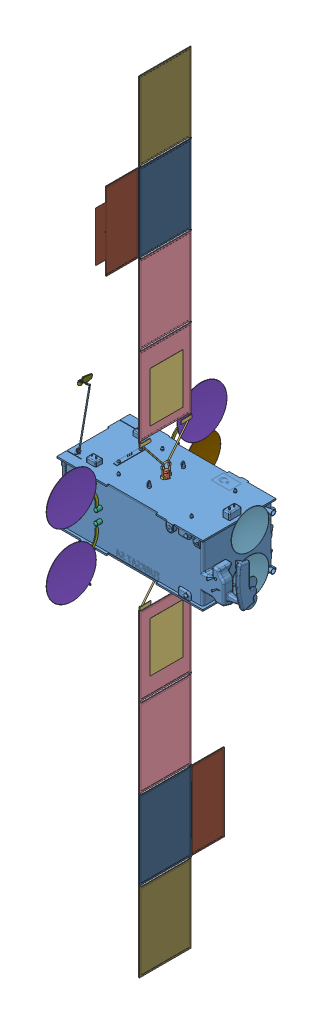
SolidWorks assembly assembly1, configuration Varsayılan. Lengths in mm.
Overall size (3700.12 16045.79 3718.83).
38 component instances, 16 part files, 76 mates.
Components (placement in the parent):
- TURKSAT_Body-1: TURKSAT_Body [Varsayılan] at (-1634.3023 1016.0246 3688.7307) size (3670 1612.58 1658.28)
- part_1-1: part_1 [Varsayılan] at (-1634.3023 1001.0246 3688.7307) x (1 0 0) z (0 1 0) size (141.09 100 150)
- solar_part_2-1: solar_part_2 [Varsayılan] at (-1640.2791 2610.2925 3688.7306) x (0 -1 0) z (0 0 1) size (2104.78 60.69 1064.93)
- SOLAR_PANEL-1: SOLAR_PANEL [Varsayılan] at (-1657.82 2695.9341 3688.7655) x (0 1 0) z (0 0 1) size (1655.94 22.5 1075)
- SOLAR_PANEL-2: SOLAR_PANEL [Varsayılan] at (-1657.82 4333.1281 3688.7655) x (0 1 0) z (0 0 1) size (1655.94 22.5 1075)
- Satelliite Dish-2: Satelliite Dish [Default] at (965.0077 812.5869 3558.7307) x (0 0 1) z (-1 0 0) size (772.34 772.34 152.2)
- Satelliite Dish-3: Satelliite Dish [Default] at (965.0077 -27.4131 3558.7307) x (0 0 1) z (-1 0 0) size (772.34 772.34 152.2)
- PART3-1: PART3 [Varsayılan] at (-2284.3023 266.0246 4368.7307) x (0.998457 0.055536 0) z (0 0 1) size (80 80 140)
- PART_2-3: PART_2 [Varsayılan] at (-2290.9418 213.9728 4968.6375) x (0.055536 -0.998457 0) z (-0.998276 -0.055526 -0.01904) size (541.67 593.01 21.9)
- SatelliiteDishBIG-5: SatelliiteDishBIG [Default] at (270.4958 -239.8039 5116.8819) x (0.017347 -0.999849 -0.000728) z (-0.999669 -0.01733 -0.019026) size (1007.37 1007.37 72.06)
- SatelliiteDish2-1: SatelliiteDish2 [Default] at (-705.909 386.0246 2167.1019) x (0 1 0) z (-0.996654 0 0.081737) size (807.67 1076.33 84.59)
- SOLAR_PANEL3-1: SOLAR_PANEL3 [Varsayılan] at (-1657.82 5970.322 3688.7655) x (0 1 0) z (0 0 1) size (1655.94 22.5 1085)
- SOLAR_PANEL3-1-2: SOLAR_PANEL3-1 [Varsayılan] at (-1657.82 5990.322 4774.6128) x (0 -1 0) z (0 0 -1) size (1597.5 17.5 883.35)
- SOLAR_PANEL4-1: SOLAR_PANEL4 [Varsayılan] at (-1657.82 7607.516 3688.7655) x (0 1 0) z (0 0 1) size (1631.25 22.5 1065)
- part_1-3: part_1 [Varsayılan] at (-1634.3023 -228.9754 3688.7307) x (-1 0 0) z (0 -1 0) size (141.09 100 150)
- solar_part_2-3: solar_part_2 [Varsayılan] at (-1640.2791 -1838.2434 3688.7309) x (0 1 0) z (0 0 -1) size (2104.78 60.69 1064.93)
- SOLAR_PANEL-5: SOLAR_PANEL [Varsayılan] at (-1657.82 -1923.8849 3688.7655) x (0 -1 0) z (0 0 -1) size (1655.94 22.5 1075)
- SOLAR_PANEL-6: SOLAR_PANEL [Varsayılan] at (-1657.82 -3561.0789 3688.7655) x (0 -1 0) z (0 0 -1) size (1655.94 22.5 1075)
- SOLAR_PANEL3-3: SOLAR_PANEL3 [Varsayılan] at (-1657.82 -5198.2729 3688.7655) x (0 -1 0) z (0 0 -1) size (1655.94 22.5 1085)
- SOLAR_PANEL4-3: SOLAR_PANEL4 [Varsayılan] at (-1657.82 -6835.4668 3688.7655) x (0 -1 0) z (0 0 -1) size (1631.25 22.5 1065)
- SOLAR_PANEL3-1-5: SOLAR_PANEL3-1 [Varsayılan] at (-1657.82 -5196.2729 3008.8359) x (0 -1 0) z (0 0 -1) size (1597.5 17.5 883.35)
- fire1-1: fire1 [Varsayılan] at (-3154.2381 1032.5795 5602.738) x (0.124128 0 -0.992266) z (0.992266 0 0.124128) size (50 76.55 20.8)
- fire_!-2: fire_! [Varsayılan] at (-2954.5343 1072.5795 4167.4546) x (-0.101949 -0.570473 0.814964) z (-0.992266 0 -0.124128) size (814.42 815.66 115)
- fire2-2: fire2 [Varsayılan] at (-3120.4869 2126.2715 3974.4156) x (0.992061 0.051434 0.11476) z (0.12216 -0.177373 -0.976533) size (185.44 52.98 60)
- fire3-1: fire3 [Varsayılan] at (-3126.1237 2097.0667 3924.7436) x (0.009481 0.1826 0.983142) z (0.029872 -0.982799 0.182248) size (291.77 72 110.83)
- SatelliiteDishBIG-10: SatelliiteDishBIG [Default] at (270.4958 1011.8531 5116.8819) x (-0.017347 -0.999849 0.000728) z (-0.999669 0.01733 -0.019026) size (1007.37 1007.37 72.06)
- PART_2-8: PART_2 [Varsayılan] at (-2290.9519 558.077 4968.6373) x (0.055536 0.998457 0) z (0.998276 -0.055526 0.01904) size (541.67 593.01 21.9)
- PART3-6: PART3 [Varsayılan] at (-2284.3023 506.0246 4368.7307) x (-0.998457 0.055536 0) z (0 0 1) size (80 80 140)
- part_1-4: part_1 [Varsayılan] at (-2284.3023 106.0246 3008.7307) x (-0.999829 0.01847 0) z (0 0 -1) size (141.09 100 150)
- PART_2-11: PART_2 [Varsayılan] at (-2279.3145 34.3175 2458.7731) x (-0.01847 -0.999829 0) z (0.99975 -0.018469 0.012623) size (541.67 593.01 21.9)
- SatelliiteDishBIG-13: SatelliiteDishBIG [Default] at (247.923 -539.2807 2390.7944) x (0.029672 0.99956 0.000141) z (-0.99948 0.029672 -0.012622) size (1007.37 1007.37 72.06)
- PART_2-12: PART_2 [Varsayılan] at (-2279.3044 737.7319 2458.7733) x (-0.01847 0.999829 0) z (-0.99975 -0.018469 -0.012623) size (541.67 593.01 21.9)
- part_1-5: part_1 [Varsayılan] at (-2284.3023 666.0246 3008.7307) x (0.999829 0.01847 0) z (0 0 -1) size (141.09 100 150)
- SatelliiteDishBIG-14: SatelliiteDishBIG [Default] at (247.923 1311.3299 2390.7944) x (-0.029672 0.99956 -0.000141) z (-0.99948 -0.029672 -0.012622) size (1007.37 1007.37 72.06)
- fire_!-4: fire_! [Varsayılan] at (-2989.2636 -300.5303 4163.1101) x (-0.101949 0.570473 0.814964) z (0.992266 0 0.124128) size (814.42 815.66 115)
- fire1-3: fire1 [Varsayılan] at (-2794.5212 -260.5303 2727.2061) x (-0.124128 0 0.992266) z (0.992266 0 0.124128) size (50 76.55 20.8)
- fire3-3: fire3 [Varsayılan] at (-3127.2551 -1303.2281 3807.4261) x (-0.009481 0.1826 -0.983142) z (0.029872 0.982799 0.182248) size (291.77 72 110.83)
- fire2-4: fire2 [Varsayılan] at (-3120.4869 -1354.2223 3974.4156) x (0.992061 -0.051434 0.11476) z (-0.12216 -0.177373 0.976533) size (185.44 52.98 60)
Mates (geometry in assembly coordinates):
- Eş Merkezli1: concentric anti-aligned: cylinder of TURKSAT_Body-1 through (-1634.3023 1001.0246 3688.7307) axis (0 1 0) radius 50; cylinder of part_1-1 through (-1634.3023 1151.0246 3688.7307) axis (0 -1 0) radius 50
- Çakışık1: coincident anti-aligned: plane of TURKSAT_Body-1 through (-1634.3023 1001.0246 3688.7307) normal (0 1 0); plane of part_1-1 through (-1634.3023 1001.0246 3688.7307) normal (0 -1 0)
- Eş Merkezli2: concentric anti-aligned: cylinder of part_1-1 through (-1634.3023 1051.0246 3548.7307) axis (0 0 1) radius 10; cylinder of solar_part_2-1 through (-1634.3023 1051.0246 3645.6287) axis (0 0 -1) radius 11.7
- Genişlik1: width aligned: plane of part_1-1 through (-1634.3023 1051.0246 3648.7307) normal (0 0 -1); plane of solar_part_2-1 through (-1634.3023 1051.0246 3728.7307) normal (0 0 1); plane of part_1-1 through (-1667.7461 1074.4246 3743.5327) normal (0 0 -1); plane of solar_part_2-1 through (-1667.7461 1074.4246 3633.9287) normal (0 0 1)
- Çakışık2: coincident aligned: plane of solar_part_2-1 through (-1661.6168 1810.5702 3156.2655) normal (0 0 -1); plane of SOLAR_PANEL-1 through (-1668.2086 -62.9763 2919.1506) normal (0 0 -1)
- Eş Merkezli4: concentric aligned: cylinder of solar_part_2-1 through (-1662.82 1877.3371 3179.6655) axis (0 0 -1) radius 8.775; cylinder of SOLAR_PANEL-1 through (-1662.82 -86.0731 2949.1506) axis (0 0 -1) radius 11.25
- Çakışık3: coincident aligned: plane of SOLAR_PANEL-1 through (-1668.2086 -62.9763 3984.1506) normal (0 0 1); plane of SOLAR_PANEL-2 through (-2512.3962 3294.7652 4221.2655) normal (0 0 1)
- Eş Merkezli5: concentric anti-aligned: cylinder of SOLAR_PANEL-1 through (-2519.8962 1308.8551 3989.1506) axis (0 0 -1) radius 7.5; cylinder of SOLAR_PANEL-2 through (-2519.8962 3272.2652 4191.2655) axis (0 0 1) radius 11.25
- Eş Merkezli8: concentric aligned: cylinder of TURKSAT_Body-1 through (-194.3023 752.5869 3558.7307) axis (1 0 0) radius 20; cylinder of Satelliite Dish-2 through (-194.3023 752.5869 3558.7307) axis (1 0 0) radius 20
- Eş Merkezli9: concentric aligned: cylinder of TURKSAT_Body-1 through (-194.3023 872.5869 3558.7307) axis (1 0 0) radius 20; cylinder of Satelliite Dish-2 through (-194.3023 872.5869 3558.7307) axis (1 0 0) radius 20
- Çakışık5: coincident anti-aligned: plane of TURKSAT_Body-1 through (-194.3023 752.5869 3558.7307) normal (1 0 0); plane of Satelliite Dish-2 through (-194.3023 812.5869 3558.7307) normal (-1 0 0)
- Eş Merkezli15: concentric anti-aligned: cylinder of TURKSAT_Body-1 through (-2284.3023 266.0246 4368.7307) axis (0 0 1) radius 40; cylinder of PART3-1 through (-2284.3023 266.0246 4488.7307) axis (0 0 -1) radius 40
- Çakışık12: coincident anti-aligned: plane of TURKSAT_Body-1 through (-2284.3023 266.0246 4368.7307) normal (0 0 1); plane of PART3-1 through (-2284.3023 266.0246 4368.7307) normal (0 0 -1)
- Eş Merkezli16: concentric anti-aligned: cylinder of PART3-1 through (-2281.5255 216.1018 4468.7307) axis (-0.055536 0.998457 0) radius 10; cylinder of PART_2-3 through (-2283.1916 246.0555 4468.7307) axis (0.055536 -0.998457 0) radius 10
- Çakışık13: coincident anti-aligned: plane of PART3-1 through (-2283.1916 246.0555 4468.7307) normal (0.055536 -0.998457 0); plane of PART_2-3 through (-2283.1916 246.0555 4468.7307) normal (-0.055536 0.998457 0)
- Eş Merkezli17: concentric anti-aligned: cylinder of PART_2-3 through (-2264.0131 -283.697 5008.0922) axis (-0.019011 -0.001057 0.999819) radius 10; cylinder of SatelliiteDishBIG-5 through (-2264.5937 -283.7293 5038.6274) axis (0.019011 0.001057 -0.999819) radius 10
- Çakışık14: coincident anti-aligned: plane of PART_2-3 through (-2264.5937 -283.7293 5038.6274) normal (-0.019011 -0.001057 0.999819); plane of SatelliiteDishBIG-5 through (-2264.5937 -283.7293 5038.6274) normal (0.019011 0.001057 -0.999819)
- Eş Merkezli18: concentric anti-aligned: cylinder of TURKSAT_Body-1 through (-2284.3023 106.0246 3008.7307) axis (0 0 -1) radius 40; cylinder of PART3-4 through (-2284.3023 106.0246 2888.7307) axis (0 0 1) radius 40
- Çakışık15: coincident anti-aligned: plane of TURKSAT_Body-1 through (-2284.3023 106.0246 3008.7307) normal (0 0 -1); plane of PART3-4 through (-2284.3023 106.0246 3008.7307) normal (0 0 1)
- Eş Merkezli19: concentric anti-aligned: cylinder of PART_2-6 through (-2264.31 105.4705 2908.7307) axis (0.999616 -0.027705 0) radius 10; cylinder of PART3-4 through (-2234.3215 104.6393 2908.7307) axis (-0.999616 0.027705 0) radius 10
- Çakışık16: coincident aligned: plane of PART_2-6 through (-2264.31 105.4705 2908.7307) normal (-0.999616 0.027705 0); circle of PART3-4
- Eş Merkezli20: concentric anti-aligned: cylinder of SatelliiteDishBIG-8 through (-2133.0387 -427.7926 2343.4356) axis (0.117683 0.050902 0.991746) radius 10; cylinder of PART_2-6 through (-1736.4298 21.6439 2373.7243) axis (-0.003552 -0.12817 -0.991746) radius 10
- Çakışık17: coincident anti-aligned: plane of SatelliiteDishBIG-8 through (-2133.0387 -427.7926 2343.4356) normal (0.117683 0.050902 0.991746); plane of PART_2-6 through (-1736.5383 17.7295 2343.4356) normal (-0.003552 -0.12817 -0.991746)
- Eş Merkezli22: concentric aligned: cylinder of TURKSAT_Body-1 through (-2284.3023 446.0246 2948.7307) axis (0 -1 0) radius 17.5; cylinder of SatelliiteDish2-1 through (-2284.3023 421.0246 2948.7307) axis (0 -1 0) radius 17.5
- Genişlik2: width aligned: plane of SatelliiteDish2-1 through (-2284.3023 351.0246 2948.7307) normal (0 -1 0); plane of TURKSAT_Body-1 through (-2284.3023 421.0246 2948.7307) normal (0 1 0); plane of SatelliiteDish2-1 through (-2284.3023 326.0246 2948.7307) normal (0 -1 0); plane of TURKSAT_Body-1 through (-1634.3023 446.0246 3688.7307) normal (0 1 0)
- Eş Merkezli23: concentric anti-aligned: cylinder of SOLAR_PANEL-2 through (-2519.8962 4909.4592 3151.2655) axis (0 0 1) radius 7.5; cylinder of SOLAR_PANEL3-1 through (-2519.8962 4909.4592 3186.2655) axis (0 0 -1) radius 7.5
- Çakışık18: coincident aligned: plane of SOLAR_PANEL-2 through (-2512.3962 3294.7652 3156.2655) normal (0 0 -1); plane of SOLAR_PANEL3-1 through (-2512.3962 4931.9592 3156.2655) normal (0 0 -1)
- Eş Merkezli24: concentric anti-aligned: cylinder of SOLAR_PANEL3-1 through (-1603.2846 5968.322 3146.1959) axis (0 1 0) radius 5; circle of SOLAR_PANEL3-1-1
- Çakışık20: coincident anti-aligned: plane of SOLAR_PANEL3-1 through (-1603.2846 5970.322 3146.1959) normal (0 1 0); plane of SOLAR_PANEL3-1-1 through (-1674.4723 1337.3544 3147.4218) normal (-0.993526 -0.10527 0.04272)
- Eş Merkezli26: concentric anti-aligned: cylinder of SOLAR_PANEL3-1 through (-2522.3962 5726.0562 4231.2655) axis (0 1 0) radius 5; cylinder of SOLAR_PANEL3-1-2 through (-2522.3962 5750.0562 4231.2655) axis (0 -1 0) radius 5
- Çakışık22: coincident anti-aligned: plane of SOLAR_PANEL3-1 through (-2522.3962 5738.0562 4231.2655) normal (0 1 0); plane of SOLAR_PANEL3-1-2 through (-2522.3962 5738.0562 4231.2655) normal (0 -1 0)
- Eş Merkezli30: concentric anti-aligned: cylinder of SOLAR_PANEL3-1 through (-2519.8962 6546.6532 3151.2655) axis (0 0 1) radius 7.5; cylinder of SOLAR_PANEL4-1 through (-2519.8962 6546.6532 3186.2655) axis (0 0 -1) radius 11.25
- Çakışık25: coincident aligned: plane of SOLAR_PANEL3-1 through (-2512.3962 4931.9592 3156.2655) normal (0 0 -1); plane of SOLAR_PANEL4-1 through (-2512.3962 6569.1532 3156.2655) normal (0 0 -1)
- Eş Merkezli31: concentric anti-aligned: cylinder of TURKSAT_Body-1 through (-1634.3023 -228.9754 3688.7307) axis (0 -1 0) radius 50; cylinder of part_1-3 through (-1634.3023 -378.9754 3688.7307) axis (0 1 0) radius 50
- Çakışık26: coincident anti-aligned: plane of TURKSAT_Body-1 through (-1634.3023 -228.9754 3688.7307) normal (0 -1 0); plane of part_1-3 through (-1634.3023 -228.9754 3688.7307) normal (0 1 0)
- Eş Merkezli32: concentric anti-aligned: cylinder of part_1-3 through (-1634.3023 -278.9754 3548.7307) axis (0 0 1) radius 10; cylinder of solar_part_2-3 through (-1634.3023 -278.9754 3645.6287) axis (0 0 -1) radius 11.7
- Genişlik3: width aligned: plane of solar_part_2-3 through (-1667.7461 -302.3754 3743.5327) normal (0 0 -1); plane of part_1-3 through (-1667.7461 -302.3754 3633.9287) normal (0 0 1); plane of solar_part_2-3 through (-1634.3023 -278.9754 3648.7307) normal (0 0 -1); plane of part_1-3 through (-1634.3023 -278.9754 3728.7307) normal (0 0 1)
- Eş Merkezli33: concentric aligned: cylinder of solar_part_2-3 through (-1662.82 -1105.2879 3179.6655) axis (0 0 -1) radius 8.775; cylinder of SOLAR_PANEL-5 through (-1662.82 -1105.2879 3186.2655) axis (0 0 -1) radius 7.5
- Çakışık27: coincident aligned: plane of solar_part_2-3 through (-1662.82 -1105.2879 3156.2655) normal (0 0 -1); plane of SOLAR_PANEL-5 through (-1655.32 -1127.7879 3156.2655) normal (0 0 -1)
- Eş Merkezli34: concentric anti-aligned: cylinder of SOLAR_PANEL-5 through (-1662.82 -2742.4819 3151.2655) axis (0 0 1) radius 7.5; cylinder of SOLAR_PANEL-6 through (-1662.82 -2742.4819 3186.2655) axis (0 0 -1) radius 7.5
- Çakışık28: coincident aligned: plane of SOLAR_PANEL-5 through (-1655.32 -1127.7879 3156.2655) normal (0 0 -1); plane of SOLAR_PANEL-6 through (-1655.32 -2764.9819 3156.2655) normal (0 0 -1)
- Eş Merkezli35: concentric anti-aligned: cylinder of SOLAR_PANEL-6 through (-1662.82 -4379.6759 3151.2655) axis (0 0 1) radius 7.5; cylinder of SOLAR_PANEL3-3 through (-1662.82 -4379.6759 3186.2655) axis (0 0 -1) radius 7.5
- Çakışık29: coincident aligned: plane of SOLAR_PANEL-6 through (-1655.32 -2764.9819 3156.2655) normal (0 0 -1); plane of SOLAR_PANEL3-3 through (-1655.32 -4402.1759 3156.2655) normal (0 0 -1)
- Eş Merkezli36: concentric anti-aligned: cylinder of SOLAR_PANEL3-3 through (-1603.2846 -5196.2729 4231.1959) axis (0 -1 0) radius 5; cylinder of SOLAR_PANEL3-1-4 through (-1962.0993 -5206.9181 4141.5308) axis (0.025863 0.999611 0.010414) radius 5
- Çakışık30: coincident anti-aligned: plane of SOLAR_PANEL3-3 through (-1603.2846 -5198.2729 4231.1959) normal (0 -1 0); plane of SOLAR_PANEL3-1-4 through (-1961.8407 -5196.922 4141.6349) normal (0.025863 0.999611 0.010414)
- Eş Merkezli38: concentric anti-aligned: cylinder of SOLAR_PANEL3-3 through (-1662.82 -6016.8698 3151.2655) axis (0 0 1) radius 7.5; cylinder of SOLAR_PANEL4-3 through (-1662.82 -6016.8698 3186.2655) axis (0 0 -1) radius 7.5
- Çakışık32: coincident aligned: plane of SOLAR_PANEL3-1-4 through (-2146.0221 -4318.1482 4056.693) normal (-0.373514 0 0.927625); plane of SOLAR_PANEL4-3
- Eş Merkezli39: concentric anti-aligned: cylinder of SOLAR_PANEL3-3 through (-1665.32 -5196.2729 3146.2655) axis (0 -1 0) radius 5; cylinder of SOLAR_PANEL3-1-5 through (-1665.32 -5208.2729 3146.2655) axis (0 1 0) radius 5
- Çakışık33: coincident aligned: plane of SOLAR_PANEL3-3 through (-1665.32 -5208.2729 3146.2655) normal (0 -1 0); plane of SOLAR_PANEL3-1-5 through (-1665.32 -5208.2729 3146.2655) normal (0 -1 0)
- Paralel1: parallel aligned: plane of solar_part_2-3 through (-1639.3242 -480.2154 3688.7307) normal (0 -1 0); plane of SOLAR_PANEL3-1-5 through (-1655.32 -5996.3559 3540.4887) normal (0 -1 0)
- Paralel2: parallel aligned: plane of SOLAR_PANEL3-3 through (-1655.32 -5999.6759 4221.2655) normal (0 -1 0); plane of SOLAR_PANEL3-1-5 through (-1655.32 -5996.3559 3540.4887) normal (0 -1 0)
- Paralel3: parallel aligned: line of SOLAR_PANEL3-3 through (-1657.82 -5999.6759 3153.2655) axis (-1 0 0); line of SOLAR_PANEL3-1-5 through (-1655.32 -5996.3559 3136.2655) axis (-1 0 0)
- Paralel4: parallel aligned: line of solar_part_2-3 through (-1621.8726 -480.2154 3601.0791) axis (-1 0 0); line of SOLAR_PANEL3-3 through (-1657.82 -5999.6759 3153.2655) axis (-1 0 0)
- Çakışık38: coincident aligned: plane of SOLAR_PANEL3-3 through (-1655.32 -4402.1759 4221.2655) normal (0 0 1); plane of SOLAR_PANEL4-3 through (-1655.32 -6039.3698 4221.2655) normal (0 0 1)
- Paralel5: parallel anti-aligned: line of SOLAR_PANEL3-1 through (-2524.8962 6528.5779 4226.2655) axis (1 0 0); line of SOLAR_PANEL3-1-2 through (-2512.3962 6545.4732 4241.2655) axis (-1 0 0)
- Paralel6: parallel anti-aligned: line of solar_part_2-1 through (-1621.8726 1252.2646 3776.3823) axis (-1 0 0); line of SOLAR_PANEL3-1 through (-2524.8962 6528.5779 4226.2655) axis (1 0 0)
- Paralel7: parallel anti-aligned: line of solar_part_2-1 through (-1610.9023 1074.4246 3774.3287) axis (-1 0 0); line of solar_part_2-3 through (-1656.7758 -421.7154 3776.3823) axis (1 0 0)
- Çakışık39: coincident anti-aligned: cylinder of TURKSAT_Body-1 through (-3028.7744 1056.0246 4139.7865) axis (0.447214 0 0.894427) radius 20; circle of fire_!-1
- Çakışık40: coincident anti-aligned: plane of TURKSAT_Body-1 through (-3028.7744 1056.0246 4139.7865) normal (0.447214 0 0.894427); plane of fire_!-1 through (-3028.7744 1056.0246 4139.7865) normal (-0.447214 0 -0.894427)
- Eş Merkezli40: concentric aligned: cylinder of fire_!-1 through (-2415.868 1898.3743 3794.2021) axis (-0.6875 0.639672 0.34375) radius 15; cylinder of fire2-1 through (-2415.9351 1898.4368 3794.2356) axis (-0.68755 0.639604 0.343775) radius 20
- Çakışık41: coincident anti-aligned: plane of fire_!-1; plane of fire2-1 through (-2415.9351 1898.4368 3794.2356) normal (0.68755 -0.639604 -0.343775)
- Eş Merkezli41: concentric aligned: cylinder of TURKSAT_Body-1 through (-2984.3023 1021.0246 4163.7307) axis (0 1 0) radius 10; cylinder of fire1-1 through (-2984.3023 1021.0246 4163.7307) axis (0 1 0) radius 10
- Çakışık42: coincident anti-aligned: plane of TURKSAT_Body-1 through (-2984.3023 1021.0246 4163.7307) normal (0 1 0); plane of fire1-1 through (-2984.3023 1021.0246 4163.7307) normal (0 -1 0)
- Çakışık43: coincident anti-aligned: cylinder of fire1-1 through (-2979.341 1072.5795 4164.3514) axis (0.992266 0 0.124128) radius 15; circle of fire_!-2
- Çakışık44: coincident anti-aligned: plane of fire1-1 through (-2979.341 1072.5795 4164.3514) normal (0.992266 0 0.124128); plane of fire_!-2 through (-2979.341 1072.5795 4164.3514) normal (-0.992266 0 -0.124128)
- Eş Merkezli42: concentric anti-aligned: cylinder of fire_!-2 through (-2984.7926 2151.9476 3966.246) axis (-0.12216 0.177373 0.976533) radius 15; cylinder of fire2-2 through (-2986.0142 2153.7213 3976.0114) axis (0.12216 -0.177373 -0.976533) radius 15
- Çakışık45: coincident anti-aligned: plane of fire_!-2 through (-2984.7926 2151.9476 3966.246) normal (-0.12216 0.177373 0.976533); plane of fire2-2 through (-2984.7926 2151.9476 3966.246) normal (0.12216 -0.177373 -0.976533)
- Eş Merkezli45: concentric anti-aligned: cylinder of fire2-2 through (-3121.0843 2145.9274 3970.7706) axis (0.029872 -0.982799 0.182248) radius 15; cylinder of fire3-1 through (-3118.6945 2067.3035 3985.3504) axis (-0.029872 0.982799 -0.182248) radius 30
- Eş Merkezli46: concentric aligned: cylinder of fire2-2 through (-3120.1881 2116.4435 3976.2381) axis (-0.029872 0.982799 -0.182248) radius 30; cylinder of fire3-1 through (-3118.6945 2067.3035 3985.3504) axis (-0.029872 0.982799 -0.182248) radius 32
- Çakışık49: coincident aligned: plane of fire2-2 through (-3120.4869 2126.2715 3974.4156) normal (-0.029872 0.982799 -0.182248); plane of fire3-1 through (-3120.4869 2126.2715 3974.4156) normal (-0.029872 0.982799 -0.182248)
- Eş Merkezli47: concentric aligned: circle of TURKSAT_Body-1; circle of part_1-4
- Çakışık50: coincident anti-aligned: plane of TURKSAT_Body-1 through (-2284.3023 106.0246 3008.7307) normal (0 0 -1); plane of part_1-4 through (-2284.3023 106.0246 3008.7307) normal (0 0 1)
- Eş Merkezli48: concentric anti-aligned: cylinder of part_1-4 through (-2286.8882 -33.9515 2958.7307) axis (0.01847 0.999829 0) radius 10; cylinder of PART_2-11 through (-2285.0411 66.0314 2958.7307) axis (-0.01847 -0.999829 0) radius 10
- Çakışık51: coincident anti-aligned: plane of part_1-4 through (-2285.0411 66.0314 2958.7307) normal (-0.01847 -0.999829 0); plane of PART_2-11 through (-2285.0411 66.0314 2958.7307) normal (0.01847 0.999829 0)
- Eş Merkezli49: concentric anti-aligned: cylinder of PART_2-11 through (-2288.0221 -464.0039 2419.3144) axis (0.012621 -0.000233 -0.99992) radius 10; cylinder of SatelliiteDishBIG-13 through (-2287.6367 -464.0111 2388.7761) axis (-0.012621 0.000233 0.99992) radius 10
- Çakışık52: coincident anti-aligned: plane of PART_2-11 through (-2287.6367 -464.0111 2388.7761) normal (0.012621 -0.000233 -0.99992); plane of SatelliiteDishBIG-13 through (-2287.6367 -464.0111 2388.7761) normal (-0.012621 0.000233 0.99992)
